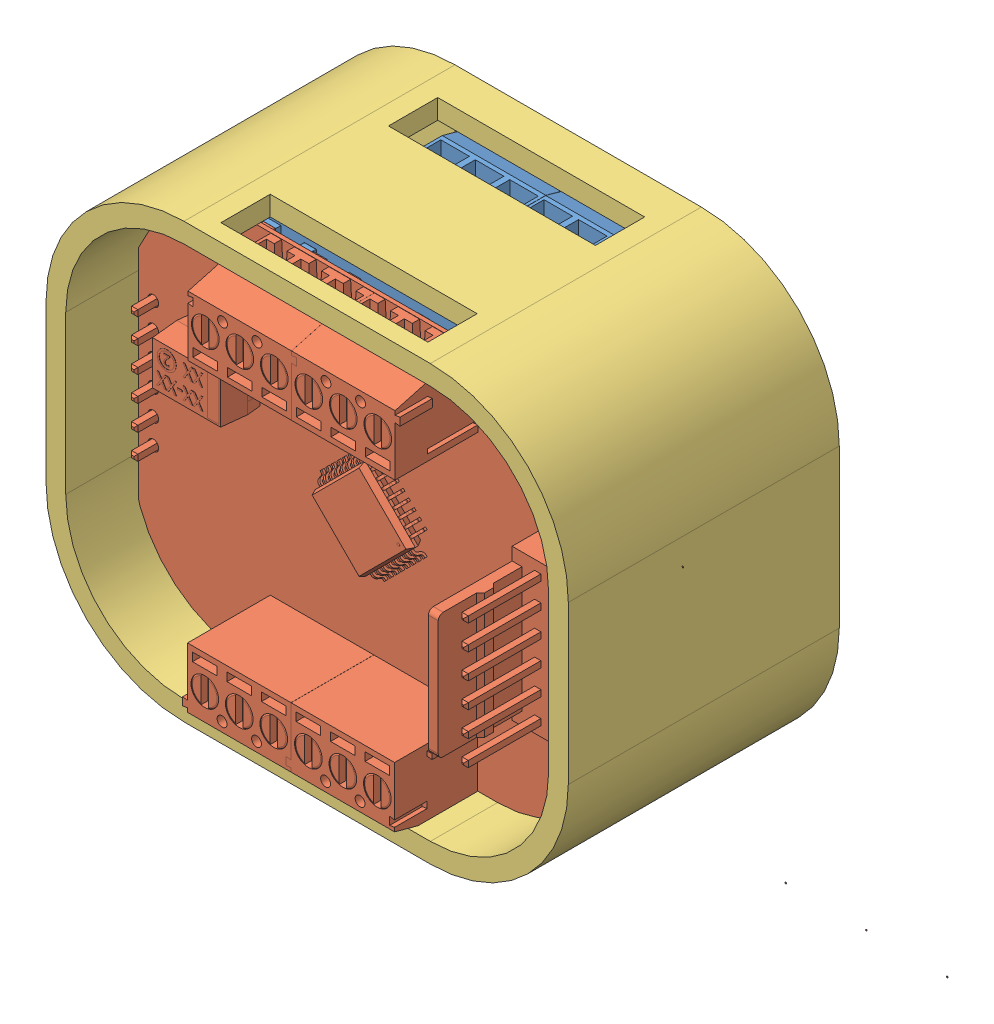
SolidWorks assembly Сборка плат смарт-бокса, configuration Default. Lengths in mm.
Overall size (85.93 44 32.41).
4 component instances, 4 part files, 9 mates.
Components (placement in the parent):
- Плата смарт-бокса 1-1: Плата смарт-бокса 1 [Default] at (-165.9192 -27.3465 18.5165) size (50.47 38.8 18.8)
- Плата смарт-бокса 2-1: Плата смарт-бокса 2 [Default] at (-116.116 -27.2195 30.3365) x (1 0 0) z (0 0 1) size (83.29 38.85 21.16)
- Корпус для смарт-бокса, новая версия-2: Корпус для смарт-бокса, новая версия [Default] at (-31.0453 -1.8751 23.405) x (1 0 0) z (0 -1 0) size (53 27.5 44)
- Смарт-бокс, крышка-1: Смарт-бокс, крышка [Default] at (-31.0453 -1.8751 37.155) x (1 0 0) z (0 -1 0) size (53 5 44) (hidden)
Mates (geometry in assembly coordinates):
- Coincident1: coincident anti-aligned: plane of Плата смарт-бокса 1-1 through (-53.5496 4.7591 26.877) normal (0 0 1); plane of Плата смарт-бокса 2-1 through (-54.7496 6.0291 26.877) normal (0 0 -1)
- Coincident2: coincident aligned: plane of Плата смарт-бокса 1-1 through (-54.7496 6.0291 18.477) normal (0 1 0); plane of Плата смарт-бокса 2-1 through (-53.4796 6.0291 28.147) normal (0 1 0)
- Coincident3: coincident aligned: plane of Плата смарт-бокса 1-1 through (-54.7496 3.4891 18.477) normal (-1 0 0); plane of Плата смарт-бокса 2-1 through (-54.7496 6.0291 29.417) normal (-1 0 0)
- Coincident9: coincident anti-aligned: plane of Корпус для смарт-бокса, новая версия-2 through (-43.5453 6.1249 37.155) normal (0 0 1); plane of Смарт-бокс, крышка-1 through (-43.5453 6.1249 37.155) normal (0 0 -1)
- Coincident10: coincident aligned: plane of Плата смарт-бокса 1-1 through (-20.5577 16.5413 9.655) normal (0 0 -1); plane of Корпус для смарт-бокса, новая версия-2 through (-43.5453 6.1249 9.655) normal (0 0 -1)
- Width2: width aligned: plane of Корпус для смарт-бокса, новая версия-2 through (-20.5453 18.1249 18.405) normal (-1 0 0); plane of Корпус для смарт-бокса, новая версия-2 through (-41.5453 18.1249 18.405) normal (1 0 0); plane of Плата смарт-бокса 1-1 through (-20.8577 11.0413 13.405) normal (-1 0 0); plane of Плата смарт-бокса 1-1 through (-41.2329 11.0634 17.305) normal (1 0 0)
- Distance2: distance = 1.75 mm: point of Плата смарт-бокса 2-1; plane of Корпус для смарт-бокса, новая версия-2 through (-43.5453 -23.8751 37.155) normal (0 -1 0)
- Coincident12: coincident aligned: plane of Корпус для смарт-бокса, новая версия-2 through (-43.5453 -23.8751 37.155) normal (0 -1 0); plane of Смарт-бокс, крышка-1 through (-43.5453 -23.8751 39.655) normal (0 -1 0)
- Coincident13: coincident aligned: plane of Корпус для смарт-бокса, новая версия-2 through (-57.5453 6.1249 37.155) normal (-1 0 0); plane of Смарт-бокс, крышка-1 through (-57.5453 6.1249 39.655) normal (-1 0 0)
